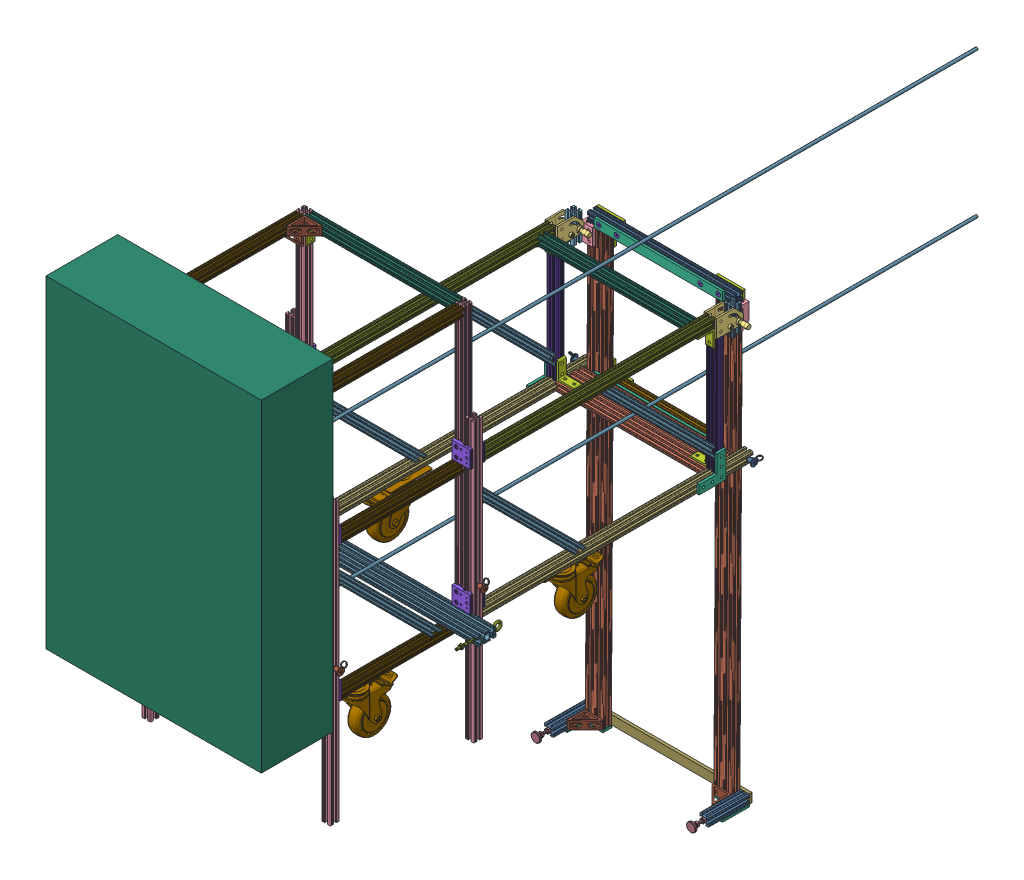
SolidWorks assembly _Tow System Assy V1.1, configuration Default. Lengths in mm. (continued)
Mates (geometry in assembly coordinates): (continued)
- Coincident1147: coincident aligned: plane of 8020 -1inch - 2 ft 3 in-13 through (-9.5504 12.7 -901.7) normal (0 1 0); plane of 8020 -1inch - 1 ft 3 in-2 through (-6.3331 12.7 190.5) normal (0 1 0)
- Coincident1148: coincident aligned: plane of 8020 -1inch - 2 ft 8 inches-1 through (-9.5504 -393.7 -215.9) normal (0 -1 0); plane of 8020 -1inch - 2 ft 7 inches-1 through (6.4164 -393.7 -212.6098) normal (0 -1 0)
- Coincident1149: coincident aligned: plane of 8020 -1inch - 2 ft 8 inches-1 through (-12.7 -371.4496 -215.9) normal (-1 0 0); plane of 8020 -1inch - 2 ft 7 inches-1 through (-12.7 393.7 -212.7504) normal (-1 0 0)
- Coincident1153: coincident anti-aligned: plane of 8020 -1inch - 1 ft 4.75 in-9 through (438.15 -374.6669 190.5) normal (0 0 -1); plane of 8020 -1inch - 1 ft 3 in-3 through (-6.4164 -390.4098 190.5) normal (0 0 1)
- Coincident1154: coincident anti-aligned: plane of 8020 -1inch - 1 ft 4.75 in-9 through (12.7 -374.5836 212.6098) normal (-1 0 0); plane of 8020 -1inch - 1 ft 3 in-3 through (12.7 -374.6669 190.5) normal (1 0 0)
- Coincident1158: coincident anti-aligned: plane of 8020 -1inch - 2 ft 8 inches-1 through (-6.4164 -390.4098 -215.9) normal (0 0 1); plane of 8020 -1inch - 2 ft 7 inches-1 through (-6.3331 393.7 -215.9) normal (0 0 -1)
- Coincident1159: coincident: plane of 8020 -1inch - 1 ft 3 in-3 through (-12.7 -371.4496 190.5) normal (-1 0 0); line of 8020 -1inch - 2 ft 8 inches-1 through (-12.7 -371.4496 -215.9) axis (0 0 -1)
- Coincident1161: coincident aligned: plane of 8020 -1inch - 2 ft 3 in-13 through (-12.7 6.3331 -901.7) normal (-1 0 0); plane of 47065T701_45 Brace - 18 in-1 through (-12.7 -47.2378 -213.673) normal (-1 0 0)
- Coincident1162: coincident aligned: plane of 8020 -1inch - 2 ft 3 in-13 through (-12.7 6.3331 -901.7) normal (-1 0 0); plane of 8020 -1inch - 1 ft 3 in-2 through (-12.7 9.5504 190.5) normal (-1 0 0)
- Coincident1164: coincident anti-aligned: plane of 47065T512_8020 - 3inch - 1 ft 4.75 in-1 through (12.7 -370.9416 -901.7) normal (-1 0 0); plane of 8020 -1inch - 2 ft 8 inches-1 through (12.7 -374.6669 -215.9) normal (1 0 0)
- Coincident1165: coincident aligned: plane of 8020 -1inch - 2 ft 3 in-13 through (6.4164 -9.4098 -215.9) normal (0 0 1); plane of 8020 -1inch - 2 ft 3 in-14 through (457.2664 -9.4098 -215.9) normal (0 0 1)
- Coincident1166: coincident aligned: plane of 8020 -1inch - 1 ft 3 in-3 through (-9.5504 -393.7 190.5) normal (0 -1 0); plane of 8020 -1inch - 2 ft 7 inches-2 through (6.4164 -393.7 193.7902) normal (0 -1 0)
- Coincident1167: coincident aligned: plane of 8020 -1inch - 1 ft 4.75 in-9 through (438.15 -387.3331 215.9) normal (0 0 1); plane of 8020 -1inch - 2 ft 7 inches-2 through (-9.5504 393.7 215.9) normal (0 0 1)
- Coincident1168: coincident anti-aligned: plane of 8020 -1inch - 1 ft 4.75 in-9 through (12.7 -374.5836 212.6098) normal (-1 0 0); plane of 8020 -1inch - 2 ft 7 inches-2 through (12.7 393.7 212.7504) normal (1 0 0)
- Coincident1169: coincident anti-aligned: plane of 47065T701_45 Brace - 18 in-1 through (-12.7 -80.9316 -215.9) normal (0 0 1); plane of 8020 -1inch - 2 ft 7 inches-1 through (-6.3331 393.7 -215.9) normal (0 0 -1)
- Coincident1170: coincident anti-aligned: plane of 8020 - 2inch - 1 ft 4.75 in-9 through (12.7 239.7749 190.5) normal (-1 0 0); plane of 8020 -1inch - 2 ft 7 inches-2 through (12.7 393.7 212.7504) normal (1 0 0)
- Coincident1171: coincident aligned: plane of 8020 - 2inch - 1 ft 4.75 in-9 through (438.15 280.5504 215.9) normal (0 0 1); plane of 8020 -1inch - 2 ft 7 inches-2 through (6.3331 393.7 215.9) normal (0 0 1)
- Coincident1175: coincident anti-aligned: plane of 8020 -1inch - 2 ft 7 inches-2 through (12.7 393.7 212.7504) normal (1 0 0); plane of 8020 - 2inch - 1 ft 4.75 in-12 through (12.7 163.5749 190.5) normal (-1 0 0)
- Coincident1176: coincident aligned: plane of 8020 -1inch - 2 ft 7 inches-2 through (6.3331 393.7 215.9) normal (0 0 1); plane of 8020 - 2inch - 1 ft 4.75 in-12 through (438.15 204.3504 215.9) normal (0 0 1)
- Coincident1178: coincident aligned: plane of 8020 -1inch - 1 ft 3 in-2 through (-6.4164 -9.4098 -190.5) normal (0 0 -1); plane of 8020 -1inch - 1 ft 3 in-3 through (-6.4164 -390.4098 -190.5) normal (0 0 -1)
- Coincident1179: coincident anti-aligned: plane of 8020 -1inch - 2 ft 7 inches-1 through (-9.5504 393.7 -190.5) normal (0 0 1); plane of 8020 -1inch - 1 ft 3 in-7 through (-6.4164 371.5902 -190.5) normal (0 0 -1)
- Coincident1180: coincident aligned: plane of 8020 -1inch - 2 ft 7 inches-1 through (-12.7 393.7 -196.8669) normal (-1 0 0); plane of 8020 -1inch - 1 ft 3 in-7 through (-12.7 390.5504 190.5) normal (-1 0 0)
- Coincident1181: coincident aligned: plane of 8020 -1inch - 2 ft 7 inches-1 through (6.4164 393.7 -212.6098) normal (0 1 0); plane of 8020 -1inch - 1 ft 3 in-7 through (-6.3331 393.7 190.5) normal (0 1 0)
- Coincident1182: coincident: plane of 8020 -1inch - 1 ft 3 in-3 through (-12.7 -371.4496 190.5) normal (-1 0 0); line of 47065T701_45 Brace - 18 in-11 through (-12.7 -54.0147 190.5) axis (0 -0.707107 -0.707107)
- Coincident1183: coincident anti-aligned: plane of 8020 -1inch - 2 ft 7 inches-2 through (-6.3331 393.7 190.5) normal (0 0 -1); plane of 47065T701_45 Brace - 18 in-11 through (-12.7 -80.9316 190.5) normal (0 0 1)
- Coincident1184: coincident anti-aligned: plane of 8020 -1inch - 1 ft 3 in-3 through (-6.3331 -368.3 190.5) normal (0 1 0); plane of 47065T701_45 Brace - 18 in-11 through (-12.7 -368.3 -96.8684) normal (0 -1 0)
- Coincident1189: coincident anti-aligned: plane of 47065T701_45 Brace - 18 in-10 through (-12.7 300.0684 190.5) normal (0 0 1); plane of 8020 -1inch - 2 ft 7 inches-2 through (-6.3331 393.7 190.5) normal (0 0 -1)
- Coincident1190: coincident anti-aligned: plane of 1 inch x 2 inch L bracket-10 through (63.5 368.3 -215.9) normal (0 1 0); plane of 8020 -1inch - 1 ft 3 in-7 through (6.3331 368.3 190.5) normal (0 -1 0)
- Coincident1191: coincident aligned: plane of 1 inch x 2 inch L bracket-10 through (12.7 322.2752 -215.9) normal (0 0 -1); plane of 8020 -1inch - 2 ft 7 inches-1 through (9.5504 393.7 -215.9) normal (0 0 -1)
- Coincident1192: coincident anti-aligned: plane of 1 inch x 2 inch L bracket-10 through (12.7 368.3 -215.9) normal (-1 0 0); plane of 8020 -1inch - 2 ft 7 inches-1 through (12.7 393.7 -209.5331) normal (1 0 0)
- Coincident1198: coincident aligned: plane of 8020 -1inch - 1 ft 3 in-2 through (-6.3331 12.7 190.5) normal (0 1 0); plane of T Bracket-25 through (19.05 12.7 190.5) normal (0 1 0)
- Coincident1199: coincident: line of 8020 -1inch - 1 ft 3 in-7 through (-6.3331 393.7 190.5) axis (0 0 -1); plane of L Bracket-19 through (12.7 393.7 222.25) normal (0 1 0)
- Coincident1200: coincident aligned: plane of 8020 -1inch - 1 ft 3 in-7 through (-12.7 390.5504 190.5) normal (-1 0 0); plane of L Bracket-19 through (-12.7 393.7 222.25) normal (-1 0 0)
- Coincident1201: coincident anti-aligned: plane of 8020 -1inch - 2 ft 7 inches-2 through (-9.5504 393.7 215.9) normal (0 0 1); plane of L Bracket-19 through (63.5 381 215.9) normal (0 0 -1)
- Coincident1204: coincident anti-aligned: plane of 8020 -1inch - 2 ft 3 in-13 through (-9.5504 12.7 -901.7) normal (0 1 0); plane of 47065T778_1 in Slider-1 through (12.7 12.7 -223.8248) normal (0 -1 0)
- Coincident1208: coincident aligned: plane of T Bracket-17 through (12.7 -393.7 -165.1) normal (0 -1 0); plane of 8020 -1inch - 2 ft 8 inches-1 through (-9.5504 -393.7 -215.9) normal (0 -1 0)
- Coincident1209: coincident anti-aligned: plane of T Bracket-17 through (12.7 -368.3 -215.9) normal (0 0 -1); plane of 8020 -1inch - 2 ft 8 inches-1 through (-6.4164 -390.4098 -215.9) normal (0 0 1)
- Coincident1212: coincident anti-aligned: plane of 47065T778_1 in Slider-1 through (-33.4772 60.198 -216.0524) normal (0 0 1); plane of 8020 -1inch - 2 ft 7 inches-3 through (-35.5431 126.825 -216.0524) normal (0 0 -1)
- Coincident1213: coincident anti-aligned: plane of 47065T778_1 in Slider-1 through (-16.51 12.7 -199.3138) normal (-1 0 0); plane of 8020 -1inch - 2 ft 7 inches-3 through (-16.51 126.825 -193.802) normal (1 0 0)
- Coincident1216: coincident aligned: plane of 8020 - 2inch - 1 ft 4.75 in-10 through (12.7 -171.2251 190.5) normal (-1 0 0); plane of 8020 - 2inch - 1 ft 4.75 in-11 through (12.7 -247.4251 190.5) normal (-1 0 0)
- Coincident1217: coincident anti-aligned: plane of T Bracket-17 through (12.7 -317.5 -203.2) normal (-1 0 0); plane of 8020 -1inch - 2 ft 7 inches-1 through (12.7 393.7 -209.5331) normal (1 0 0)
- Coincident1221: coincident anti-aligned: plane of 8020 -1inch - 1 ft 2 in-1 through (-12.7 -12.7 -923.9504) normal (-1 0 0); plane of L Bracket-17 through (-12.7 -317.5 -914.4) normal (1 0 0)
- Coincident1222: coincident aligned: plane of 8020 -1inch - 1 ft 2 in-1 through (-9.5504 -12.7 -901.7) normal (0 0 1); plane of L Bracket-17 through (-19.05 -317.5 -901.7) normal (0 0 1)
- Coincident1223: coincident aligned: plane of L Bracket-17 through (-19.05 -368.3 -851.3) normal (0 1 0); plane of 8020 -1inch - 2 ft 8 inches-1 through (-6.3331 -368.3 -215.9) normal (0 1 0)
- Coincident1224: coincident aligned: line of 8020 -1inch - 1 ft 3 in-3 through (-6.3331 -368.3 190.5) axis (0 0 -1); line of 8020 -1inch - 2 ft 8 inches-1 through (-6.3331 -368.3 -215.9) axis (0 0 -1)
- Coincident1225: coincident aligned: plane of 8020 -1inch - 2 ft 3 in-13 through (6.4164 -9.4098 -215.9) normal (0 0 1); plane of 8020 -1inch - 2 ft 8 inches-2 through (444.4336 -390.4098 -215.9) normal (0 0 1)
- Coincident1226: coincident anti-aligned: plane of 47065T701_45 Brace - 18 in-2 through (438.15 -368.3 -96.8684) normal (0 -1 0); plane of 8020 -1inch - 2 ft 8 inches-2 through (460.4004 -368.3 -215.9) normal (0 1 0)
- Coincident1227: coincident anti-aligned: plane of 8020 -1inch - 1 ft 3 in-2 through (12.7 6.3331 190.5) normal (1 0 0); plane of T Bracket-25 through (12.7 0 139.7) normal (-1 0 0)
- Coincident1228: coincident aligned: plane of 8020 -1inch - 2 ft 7 inches-2 through (9.5504 393.7 190.5) normal (0 0 -1); plane of T Bracket-25 through (19.05 38.1 190.5) normal (0 0 -1)
- Coincident1230: coincident anti-aligned: plane of 8020 -1inch - 1 ft 3 in-3 through (12.7 -374.6669 190.5) normal (1 0 0); plane of 47065T736_ Interior 90 guesset for 1 in-3 through (12.7 -390.525 190.5) normal (-1 0 0)
- Coincident1231: coincident anti-aligned: plane of 8020 -1inch - 1 ft 4.75 in-9 through (438.15 -374.6669 190.5) normal (0 0 -1); plane of 47065T736_ Interior 90 guesset for 1 in-3 through (63.5 -390.525 190.5) normal (0 0 1)
- Coincident1232: coincident aligned: plane of 8020 -1inch - 1 ft 4.75 in-9 through (438.15 -368.3 193.6496) normal (0 1 0); plane of 47065T736_ Interior 90 guesset for 1 in-3 through (15.4972 -368.3 144.4752) normal (0 1 0)
- Coincident1233: coincident aligned: plane of 8020 - 2inch - 1 ft 4.75 in-10 through (438.15 -155.8496 215.9) normal (0 0 1); plane of 8020 - 2inch - 1 ft 4.75 in-11 through (438.15 -206.6496 215.9) normal (0 0 1)
- Coincident1235: coincident aligned: plane of 8020 - 2inch - 1 ft 4.75 in-9 through (12.7 239.7749 190.5) normal (-1 0 0); plane of 8020 - 2inch - 1 ft 4.75 in-10 through (12.7 -171.2251 190.5) normal (-1 0 0)
- Coincident1239: coincident anti-aligned: plane of 8020 -1inch - 1 ft 3 in-2 through (-6.3331 12.7 190.5) normal (0 1 0); plane of 47065T778_1 in Slider-4 through (12.7 12.7 223.8248) normal (0 -1 0)
- Coincident1242: coincident: line of 8020 -1inch - 1 ft 3 in-3 through (-6.3331 -368.3 190.5) axis (0 0 -1); plane of 47065T778_1 in Slider-3 through (12.7 -368.3 223.8248) normal (0 -1 0)
- Coincident1243: coincident anti-aligned: plane of 8020 -1inch - 2 ft 7 inches-5 through (-38.7604 126.825 216.0524) normal (0 0 1); plane of 47065T778_1 in Slider-4 through (-33.4772 12.827 216.0524) normal (0 0 -1)
- Coincident1244: coincident anti-aligned: plane of 8020 -1inch - 2 ft 7 inches-5 through (-16.51 126.825 212.9028) normal (1 0 0); plane of 47065T778_1 in Slider-4 through (-16.51 12.7 193.2686) normal (-1 0 0)
- Coincident1245: coincident aligned: plane of 8020 -1inch - 2 ft 7 inches-3 through (-22.7936 126.825 -212.7622) normal (0 1 0); plane of 8020 -1inch - 2 ft 7 inches-5 through (-22.7936 126.825 193.9426) normal (0 1 0)
- Coincident1247: coincident anti-aligned: plane of 8020 -1inch - 2 ft 7 inches-1 through (-9.5504 393.7 -190.5) normal (0 0 1); plane of 47065T736_ Interior 90 guesset for 1 in-4 through (-12.7 368.3 -190.5) normal (0 0 -1)
- Coincident1248: coincident anti-aligned: plane of 8020 -1inch - 1 ft 3 in-7 through (-9.5504 368.3 190.5) normal (0 -1 0); plane of 47065T736_ Interior 90 guesset for 1 in-4 through (-12.7 368.3 -139.7) normal (0 1 0)
- Coincident1249: coincident aligned: plane of 8020 -1inch - 1 ft 3 in-7 through (-12.7 374.6669 190.5) normal (-1 0 0); plane of 47065T736_ Interior 90 guesset for 1 in-4 through (-12.7 322.2752 -187.7028) normal (-1 0 0)
- Distance48: distance = 140 mm aligned: plane of 8020 - 2inch - 1 ft 4.75 in-10 through (438.15 -127.3 193.6496) normal (0 1 0); plane of 8020 -1inch - 2 ft 3 in-14 through (441.2996 12.7 -901.7) normal (0 1 0)
- Coincident1252: coincident aligned: plane of 8020 -1inch - 2 ft 3 in-14 through (463.55 9.5504 -901.7) normal (1 0 0); plane of 8020 -1inch - 1 ft 3 in-6 through (463.55 6.3331 190.5) normal (1 0 0)
- Coincident1255: coincident: plane of 8020 -1inch - 1 ft 3 in-3 through (-6.4164 -390.4098 -190.5) normal (0 0 -1); line of 8020 -1inch - 2 ft 7 inches-1 through (-9.5504 393.7 -190.5) axis (0 -1 0)
- Coincident1256: coincident anti-aligned: plane of 8020 -1inch - 1 ft 4.75 in-9 through (438.15 -374.6669 190.5) normal (0 0 -1); plane of 8020 -1inch - 1 ft 3 in-4 through (444.4336 -390.4098 190.5) normal (0 0 1)
- Coincident1257: coincident anti-aligned: plane of 8020 -1inch - 1 ft 4.75 in-9 through (438.15 -374.5836 212.6098) normal (1 0 0); plane of 8020 -1inch - 1 ft 3 in-4 through (438.15 -371.4496 190.5) normal (-1 0 0)
- Coincident1258: coincident aligned: plane of 8020 -1inch - 1 ft 3 in-4 through (444.4336 -390.4098 190.5) normal (0 0 1); plane of 8020 -1inch - 1 ft 3 in-6 through (444.4336 -9.4098 190.5) normal (0 0 1)
- Coincident1260: coincident aligned: plane of 8020 -1inch - 1 ft 3 in-4 through (463.55 -374.6669 190.5) normal (1 0 0); plane of 8020 -1inch - 2 ft 8 inches-2 through (463.55 -374.6669 -215.9) normal (1 0 0)
- Coincident1261: coincident: line of 8020 -1inch - 1 ft 3 in-4 through (463.55 -371.4496 190.5) axis (0 0 -1); plane of 47065T701_45 Brace - 18 in-2 through (463.55 -60.7441 206.2333) normal (1 0 0)
- Coincident1262: coincident aligned: plane of 8020 -1inch - 1 ft 3 in-4 through (444.4336 -390.4098 190.5) normal (0 0 1); plane of 47065T701_45 Brace - 18 in-2 through (438.15 -80.9316 190.5) normal (0 0 1)
- Coincident1263: coincident aligned: plane of 8020 -1inch - 2 ft 3 in-14 through (457.1831 12.7 -901.7) normal (0 1 0); plane of 8020 -1inch - 1 ft 3 in-6 through (460.4004 12.7 190.5) normal (0 1 0)
- Coincident1265: coincident: line of 8020 -1inch - 2 ft 8 inches-2 through (463.55 -371.4496 -215.9) axis (0 0 -1); plane of 47065T701_45 Brace - 18 in-12 through (463.55 -49.5128 -211.398) normal (1 0 0)
- Coincident1266: coincident anti-aligned: plane of 8020 -1inch - 2 ft 8 inches-2 through (460.4004 -368.3 -215.9) normal (0 1 0); plane of 47065T701_45 Brace - 18 in-12 through (438.15 -368.3 -503.2684) normal (0 -1 0)
- Coincident1267: coincident aligned: plane of 8020 -1inch - 2 ft 8 inches-2 through (444.4336 -390.4098 -215.9) normal (0 0 1); plane of 47065T701_45 Brace - 18 in-12 through (438.15 -80.9316 -215.9) normal (0 0 1)
- Distance49: distance = 110 mm aligned: plane of 8020 - 2inch - 1 ft 4.75 in-9 through (438.15 283.7 209.5331) normal (0 1 0); plane of 8020 -1inch - 2 ft 7 inches-2 through (6.4164 393.7 193.7902) normal (0 1 0)
- Coincident1269: coincident anti-aligned: plane of 8020 -1inch - 1 ft 3 in-7 through (12.7 387.3331 190.5) normal (1 0 0); plane of 8020 -1inch - 1 ft 4.75 in-20 through (12.7 387.4164 212.6098) normal (-1 0 0)
- Coincident1270: coincident aligned: plane of 8020 -1inch - 1 ft 3 in-7 through (9.5504 393.7 190.5) normal (0 1 0); plane of 8020 -1inch - 1 ft 4.75 in-20 through (438.15 393.7 209.5331) normal (0 1 0)
- Coincident1272: coincident anti-aligned: plane of 8020 -1inch - 1 ft 3 in-7 through (-6.4164 371.5902 190.5) normal (0 0 1); plane of 8020 -1inch - 1 ft 4.75 in-20 through (438.15 387.3331 190.5) normal (0 0 -1)
- Coincident1273: coincident anti-aligned: plane of 8020 -1inch - 1 ft 3 in-7 through (-6.4164 371.5902 -190.5) normal (0 0 -1); plane of 8020 -1inch - 1 ft 4.75 in-19 through (438.15 390.5504 -190.5) normal (0 0 1)
- Coincident1274: coincident aligned: plane of 8020 -1inch - 1 ft 3 in-7 through (9.5504 393.7 190.5) normal (0 1 0); plane of 8020 -1inch - 1 ft 4.75 in-19 through (438.15 393.7 -196.8669) normal (0 1 0)
- Coincident1275: coincident anti-aligned: plane of 8020 -1inch - 1 ft 3 in-7 through (12.7 387.3331 190.5) normal (1 0 0); plane of 8020 -1inch - 1 ft 4.75 in-19 through (12.7 387.4164 -193.7902) normal (-1 0 0)
- Coincident1276: coincident anti-aligned: plane of 8020 -1inch - 1 ft 2 in-2 through (463.55 -12.7 -904.8496) normal (1 0 0); plane of L Bracket-18 through (463.55 -381 -850.9) normal (-1 0 0)
- Coincident1277: coincident aligned: plane of 8020 -1inch - 2 ft 8 inches-2 through (460.4004 -368.3 -215.9) normal (0 1 0); plane of L Bracket-18 through (469.9 -368.3 -850.9) normal (0 1 0)
- Coincident1278: coincident anti-aligned: plane of 47065T512_8020 - 3inch - 1 ft 4.75 in-1 through (12.7 -368.3 -904.8496) normal (0 1 0); plane of 1 inch x 2 inch L bracket-44 through (63.5 -368.3 -904.875) normal (0 -1 0)
- Coincident1279: coincident anti-aligned: plane of 47065T512_8020 - 3inch - 1 ft 4.75 in-1 through (12.7 -368.3 -904.8496) normal (0 1 0); plane of 1 inch x 2 inch L bracket-45 through (387.35 -368.3 -927.1) normal (0 -1 0)
- Coincident1280: coincident anti-aligned: plane of 8020 -1inch - 1 ft 3 in-7 through (12.7 387.3331 190.5) normal (1 0 0); plane of 47065T736_ Interior 90 guesset for 1 in-5 through (12.7 371.475 -139.7) normal (-1 0 0)
- Coincident1281: coincident aligned: plane of 8020 -1inch - 1 ft 3 in-7 through (-6.3331 393.7 190.5) normal (0 1 0); plane of 47065T736_ Interior 90 guesset for 1 in-5 through (58.7248 393.7 -187.7028) normal (0 1 0)
- Coincident1282: coincident anti-aligned: plane of 8020 -1inch - 1 ft 4.75 in-19 through (438.15 390.5504 -190.5) normal (0 0 1); plane of 47065T736_ Interior 90 guesset for 1 in-5 through (12.7 371.475 -190.5) normal (0 0 -1)
- Coincident1283: coincident aligned: plane of 8020 -1inch - 2 ft 7 inches-1 through (6.4164 393.7 -212.6098) normal (0 1 0); plane of 8020 -1inch - 2 ft 7 inches-6 through (457.2664 393.7 -212.6098) normal (0 1 0)
- Coincident1284: coincident: line of 8020 -1inch - 2 ft 7 inches-1 through (-6.3331 393.7 -215.9) axis (0 -1 0); plane of 8020 -1inch - 2 ft 7 inches-6 through (444.5169 393.7 -215.9) normal (0 0 -1)
- Coincident1285: coincident anti-aligned: plane of 8020 -1inch - 1 ft 4.75 in-19 through (438.15 387.4164 -193.7902) normal (1 0 0); plane of 8020 -1inch - 2 ft 7 inches-6 through (438.15 393.7 -212.7504) normal (-1 0 0)
- Coincident1286: coincident aligned: plane of 8020 -1inch - 2 ft 7 inches-6 through (457.2664 393.7 -212.6098) normal (0 1 0); plane of 8020 -1inch - 2 ft 7 inches-8 through (457.2664 393.7 193.7902) normal (0 1 0)
- Coincident1287: coincident aligned: plane of 8020 -1inch - 2 ft 7 inches-6 through (463.55 393.7 -209.5331) normal (1 0 0); plane of 8020 -1inch - 2 ft 7 inches-8 through (463.55 393.7 196.8669) normal (1 0 0)
- Coincident1288: coincident aligned: plane of 8020 -1inch - 1 ft 4.75 in-20 through (438.15 387.3331 190.5) normal (0 0 -1); plane of 8020 -1inch - 2 ft 7 inches-8 through (444.5169 393.7 190.5) normal (0 0 -1)
- Coincident1289: coincident aligned: plane of 8020 -1inch - 1 ft 4.75 in-20 through (438.15 393.7 193.6496) normal (0 1 0); plane of 8020 -1inch - 1 ft 3 in-8 through (444.5169 393.7 190.5) normal (0 1 0)
- Coincident1290: coincident anti-aligned: plane of 8020 -1inch - 1 ft 4.75 in-20 through (438.15 387.4164 212.6098) normal (1 0 0); plane of 8020 -1inch - 1 ft 3 in-8 through (438.15 390.5504 190.5) normal (-1 0 0)
- Coincident1291: coincident anti-aligned: plane of 8020 -1inch - 1 ft 4.75 in-20 through (438.15 387.3331 190.5) normal (0 0 -1); plane of 8020 -1inch - 1 ft 3 in-8 through (444.4336 371.5902 190.5) normal (0 0 1)
- Coincident1294: coincident anti-aligned: plane of 8020 -1inch - 2 ft 3 in-14 through (457.1831 12.7 -901.7) normal (0 1 0); plane of 47065T778_1 in Slider-6 through (438.15 12.7 -223.8248) normal (0 -1 0)
- Coincident1301: coincident anti-aligned: plane of 8020 -1inch - 1 ft 3 in-6 through (460.4004 12.7 190.5) normal (0 1 0); plane of 47065T778_1 in Slider-8 through (438.15 12.7 182.5752) normal (0 -1 0)
- Coincident1304: coincident anti-aligned: plane of 8020 -1inch - 1 ft 3 in-4 through (460.4004 -368.3 190.5) normal (0 1 0); plane of 47065T778_1 in Slider-7 through (438.15 -368.3 223.8248) normal (0 -1 0)
- Coincident1305: coincident anti-aligned: plane of 8020 -1inch - 2 ft 7 inches-7 through (470.5096 126.825 216.0524) normal (0 0 1); plane of 47065T778_1 in Slider-8 through (484.3272 60.198 216.0524) normal (0 0 -1)
- Coincident1306: coincident anti-aligned: plane of 8020 -1inch - 2 ft 7 inches-7 through (467.36 126.825 209.6855) normal (-1 0 0); plane of 47065T778_1 in Slider-8 through (467.36 12.7 213.1314) normal (1 0 0)
- Coincident1307: coincident aligned: plane of 8020 -1inch - 2 ft 7 inches-5 through (-22.7936 126.825 193.9426) normal (0 1 0); plane of 8020 -1inch - 2 ft 7 inches-7 through (486.4764 126.825 193.9426) normal (0 1 0)
- Coincident1308: coincident anti-aligned: plane of 47065T778_1 in Slider-6 through (484.3272 60.198 -190.3476) normal (0 0 -1); plane of 8020 -1inch - 2 ft 7 inches-9 through (470.5096 126.825 -190.3476) normal (0 0 1)
- Coincident1309: coincident anti-aligned: plane of 47065T778_1 in Slider-6 through (467.36 12.7 -193.2686) normal (1 0 0); plane of 8020 -1inch - 2 ft 7 inches-9 through (467.36 126.825 -196.7145) normal (-1 0 0)
- Coincident1310: coincident aligned: plane of 8020 -1inch - 2 ft 7 inches-7 through (486.4764 126.825 193.9426) normal (0 1 0); plane of 8020 -1inch - 2 ft 7 inches-9 through (486.4764 126.825 -212.4574) normal (0 1 0)
- Coincident1313: coincident aligned: plane of 8020 -1inch - 1 ft 3 in-2 through (0 0 0) normal (0 0 1)
- Coincident1314: coincident aligned: plane of 8020 -1inch - 1 ft 3 in-2 through (0 0 0) normal (0 1 0)
- Coincident1315: coincident aligned: plane of 8020 -1inch - 1 ft 3 in-2 through (0 0 0) normal (1 0 0)
- Coincident1316: coincident aligned: plane of 8020 -1inch - 415mm-1 through (433.1224 9.4721 -1008.3493) normal (0 0.999985 -0.005452); plane of T Bracket-24 through (94.3224 9.4203 -1017.8488) normal (0 0.999985 -0.005452)
- Coincident1317: coincident aligned: plane of 8020 -1inch - 415mm-1 through (433.1224 9.4721 -1008.3493) normal (0 0.999985 -0.005452); plane of T Bracket-23 through (432.7276 9.4203 -1017.8488) normal (0 0.999985 -0.005452)
- Coincident1318: coincident aligned: plane of 47065T125_2inch - 4 ft-1 through (18.1224 -15.9275 -1008.2108) normal (-1 0 0); plane of 8020 -1inch - 415mm-1 through (18.1224 -12.5503 -992.2622) normal (-1 0 0)
- Coincident1321: coincident anti-aligned: plane of T Bracket-25 through (19.05 12.7 139.7) normal (0 0 -1); plane of 47065T237_8020 2 in interior corner bracket-1 through (-7.9248 20.6375 139.7) normal (0 0 1)
- Coincident1322: coincident aligned: plane of 8020 -1inch - 1 ft 3 in-2 through (12.7 -9.5504 190.5) normal (1 0 0); plane of 47065T237_8020 2 in interior corner bracket-1 through (12.7 46.0375 139.7) normal (1 0 0)
- Coincident1323: coincident anti-aligned: plane of 47065T237_8020 2 in interior corner bracket-1 through (12.7 20.6375 139.7) normal (0 -1 0); plane of 1614T644_1in x 48mm Aluminium bar - 5_16 thick-1 through (12.7 20.6375 140.075) normal (0 1 0)
- Coincident1324: coincident aligned: plane of 47065T237_8020 2 in interior corner bracket-1 through (-7.9248 20.6375 92.075) normal (0 0 -1); plane of 1614T644_1in x 48mm Aluminium bar - 5_16 thick-1 through (0 16.6687 92.075) normal (0 0 -1)
- Coincident1325: coincident aligned: plane of 47065T237_8020 2 in interior corner bracket-1 through (12.7 46.0375 139.7) normal (1 0 0); plane of 1614T644_1in x 48mm Aluminium bar - 5_16 thick-1 through (12.7 20.6375 140.075) normal (1 0 0)
- Coincident1326: coincident anti-aligned: plane of 8020 -1inch - 1 ft 3 in-2 through (9.5504 12.7 190.5) normal (0 1 0); plane of 1614T644_1in x 48mm Aluminium bar - 5_16 thick-1 through (12.7 12.7 140.075) normal (0 -1 0)
- Coincident1329: coincident aligned: plane of 8020 - 2inch - 1 ft 4.75 in-10 through (438.15 -130.4496 215.9) normal (0 0 1); plane of 8020 - 2inch - 1 ft 4.75 in-12 through (438.15 204.3504 215.9) normal (0 0 1)
- Coincident1334: coincident anti-aligned: plane of 8020 -1inch - 2 ft 8 inches-1 through (-9.5504 -393.7 -215.9) normal (0 -1 0); plane of 5537T435_ Caster Wheel 265lb Cap-1 through (-1.2 -393.7 -479.1893) normal (0 1 0)
- Coincident1335: coincident aligned: plane of 8020 -1inch - 2 ft 8 inches-1 through (-12.7 -387.3331 -215.9) normal (-1 0 0); plane of 5537T435_ Caster Wheel 265lb Cap-1 through (-12.7 -393.7 -505.2661) normal (-1 0 0)
- Coincident1336: coincident: line of 47065T701_45 Brace - 18 in-1 through (-6.3331 -368.2999 -539.1893) axis (-1 0 0); plane of 5537T435_ Caster Wheel 265lb Cap-1 through (27.3 -393.7 -539.1893) normal (0 0 -1)
- Coincident1337: coincident aligned: plane of 8020 -1inch - 1 ft 3 in-3 through (-12.7 -387.3331 190.5) normal (-1 0 0); plane of 5537T435_ Caster Wheel 265lb Cap-2 through (-12.7 -393.7 54.4232) normal (-1 0 0)
- Coincident1338: coincident anti-aligned: plane of 8020 -1inch - 1 ft 3 in-3 through (-9.5504 -393.7 190.5) normal (0 -1 0); plane of 5537T435_ Caster Wheel 265lb Cap-2 through (-1.2 -393.7 80.5) normal (0 1 0)
- Distance51: distance = 50 mm aligned: plane of 5537T435_ Caster Wheel 265lb Cap-2 through (27.3 -393.7 140.5) normal (0 0 1); plane of 8020 -1inch - 1 ft 3 in-3 through (-6.4164 -390.4098 190.5) normal (0 0 1)
- Coincident1340: coincident anti-aligned: plane of 8020 -1inch - 1 ft 3 in-4 through (457.1831 -393.7 190.5) normal (0 -1 0); plane of 5537T435_ Caster Wheel 265lb Cap-4 through (452.05 -393.7 105.1) normal (0 1 0)
- Coincident1341: coincident anti-aligned: plane of 8020 -1inch - 2 ft 8 inches-2 through (457.1831 -393.7 -215.9) normal (0 -1 0); plane of 5537T435_ Caster Wheel 265lb Cap-3 through (452.05 -393.7 -479.1893) normal (0 1 0)
- Coincident1342: coincident aligned: plane of 8020 -1inch - 2 ft 8 inches-2 through (463.55 -374.6669 -215.9) normal (1 0 0); plane of 5537T435_ Caster Wheel 265lb Cap-3 through (463.55 -393.7 -539.1893) normal (1 0 0)
- Coincident1343: coincident: line of 47065T701_45 Brace - 18 in-12 through (460.4004 -368.2999 -539.1893) axis (-1 0 0); plane of 5537T435_ Caster Wheel 265lb Cap-3 through (423.55 -393.7 -539.1893) normal (0 0 -1)
- Coincident1344: coincident aligned: plane of 8020 -1inch - 1 ft 3 in-4 through (463.55 -390.5504 190.5) normal (1 0 0); plane of 5537T435_ Caster Wheel 265lb Cap-4 through (463.55 -393.7 131.1768) normal (1 0 0)
- Distance52: distance = 25.4 mm anti-aligned: plane of 5537T435_ Caster Wheel 265lb Cap-4 through (423.55 -393.7 165.1) normal (0 0 1); plane of 8020 -1inch - 2 ft 7 inches-8 through (460.4004 393.7 190.5) normal (0 0 -1)
- Distance55: distance = 25.4 mm anti-aligned: plane of L Bracket-19 through (63.5 381 222.25) normal (0 0 1); plane of Electrical Enclosure Placeholder-1 through (-77.7 -393.7 247.65) normal (0 0 -1)
- Coincident1348: coincident aligned: plane of 8020 -1inch - 1 ft 4.75 in-9 through (438.15 -393.7 212.7504) normal (0 -1 0); plane of Electrical Enclosure Placeholder-1 through (-77.7 -393.7 450.85) normal (0 -1 0)
- Distance53: distance = 65 mm aligned: plane of Electrical Enclosure Placeholder-1 through (-77.7 -393.7 450.85) normal (-1 0 0); plane of 8020 -1inch - 2 ft 7 inches-2 through (-12.7 393.7 209.5331) normal (-1 0 0)
- Concentric49: concentric anti-aligned: cylinder of 8020 -1inch - 2 ft 7 inches-2 through (12.7 -279.4 203.2) axis (-1 0 0) radius 3.175; cylinder of 92851A125_SS HIGH-TENSION PUSH-BUTTON QUICK-RELEASE PIN - 2in length-2 through (-62.5475 -279.4 203.2) axis (1 0 0) radius 3.1559
- Coincident1351: coincident anti-aligned: plane of 8020 -1inch - 2 ft 7 inches-5 through (-41.91 126.825 193.802) normal (-1 0 0); plane of 92851A125_SS HIGH-TENSION PUSH-BUTTON QUICK-RELEASE PIN - 2in length-2 through (-41.91 -275.3286 200.577) normal (1 0 0)
- Concentric50: concentric aligned: cylinder of 8020 -1inch - 2 ft 7 inches-6 through (463.55 -279.4 -203.2) axis (-1 0 0) radius 3.175; cylinder of 92851A125_SS HIGH-TENSION PUSH-BUTTON QUICK-RELEASE PIN - 2in length-4 through (513.3975 -279.4 -203.2) axis (-1 0 0) radius 3.1559
- Coincident1353: coincident anti-aligned: plane of 8020 -1inch - 2 ft 7 inches-9 through (492.76 126.825 -209.3807) normal (1 0 0); plane of 92851A125_SS HIGH-TENSION PUSH-BUTTON QUICK-RELEASE PIN - 2in length-4 through (492.76 -283.9092 -201.4325) normal (-1 0 0)
- Concentric51: concentric aligned: cylinder of 8020 -1inch - 2 ft 7 inches-8 through (463.55 -279.4 203.2) axis (-1 0 0) radius 3.175; cylinder of 92851A125_SS HIGH-TENSION PUSH-BUTTON QUICK-RELEASE PIN - 2in length-3 through (513.3975 -279.4 203.2) axis (-1 0 0) radius 3.1559
- Coincident1354: coincident anti-aligned: plane of 8020 -1inch - 2 ft 7 inches-7 through (492.76 126.825 197.0193) normal (1 0 0); plane of 92851A125_SS HIGH-TENSION PUSH-BUTTON QUICK-RELEASE PIN - 2in length-3 through (492.76 -283.325 206.0374) normal (-1 0 0)
- Coincident1355: coincident anti-aligned: plane of 8020 -1inch - 2 ft 7 inches-3 through (-41.91 126.825 -212.9028) normal (-1 0 0); plane of 92851A125_SS HIGH-TENSION PUSH-BUTTON QUICK-RELEASE PIN - 2in length-1 through (-41.91 -277.9317 -198.5847) normal (1 0 0)
- Coincident1356: coincident anti-aligned: plane of 8020 -1inch - 2 ft 7 inches-1 through (6.3331 393.7 -190.5) normal (0 0 1); plane of 8020 - 2inch - 2 ft 2 in-1 through (-104.775 -346.0496 -190.5) normal (0 0 -1)
- Coincident1357: coincident anti-aligned: plane of 8020 -1inch - 1 ft 3 in-3 through (-6.3331 -368.3 190.5) normal (0 1 0); plane of 8020 - 2inch - 2 ft 2 in-1 through (-104.775 -368.3 -187.3504) normal (0 -1 0)
- Concentric54: concentric aligned: cylinder of 8020 - 2inch - 2 ft 2 in-1 through (542.925 -355.6 -139.7) axis (0 0 -1) radius 4.445; cylinder of 3032T610_316 SS EYEBOLT W NUT 1-4_20 x 4 in-1 through (542.925 -355.6 -88.9) axis (0 0 -1) radius 3.175
- Coincident1363: coincident anti-aligned: plane of 8020 - 2inch - 2 ft 2 in-1 through (-104.775 -346.0496 -190.5) normal (0 0 -1); plane of 3032T610_316 SS EYEBOLT W NUT 1-4_20 x 4 in-1 through (542.925 -350.8375 -190.5) normal (0 0 1)
- Parallel19: parallel aligned: plane of 8020 - 2inch - 2 ft 2 in-1 through (-104.775 -342.9 -142.8496) normal (0 1 0); plane of 3032T610_316 SS EYEBOLT W NUT 1-4_20 x 4 in-1 through (546.1329 -350.0437 -101.6) normal (0 1 0)
- Concentric55: concentric aligned: cylinder of 8020 - 2inch - 2 ft 2 in-1 through (-92.075 -355.6 -139.7) axis (0 0 -1) radius 4.445; cylinder of 3032T610_316 SS EYEBOLT W NUT 1-4_20 x 4 in-2 through (-92.075 -355.6 -88.9) axis (0 0 -1) radius 3.175
- Coincident1365: coincident anti-aligned: plane of 8020 - 2inch - 2 ft 2 in-1 through (-104.775 -346.0496 -190.5) normal (0 0 -1); plane of 3032T610_316 SS EYEBOLT W NUT 1-4_20 x 4 in-2 through (-92.075 -350.8375 -190.5) normal (0 0 1)
- Parallel20: parallel aligned: plane of 8020 - 2inch - 2 ft 2 in-1 through (-104.775 -342.9 -142.8496) normal (0 1 0); plane of 3032T610_316 SS EYEBOLT W NUT 1-4_20 x 4 in-2 through (-88.8671 -350.0437 -101.6) normal (0 1 0)
- Coincident1367: coincident anti-aligned: plane of 8020 - 2inch - 2 ft 2 in-1 through (-104.775 -342.9 -184.1331) normal (0 1 0); plane of 47065T778_1 in Slider-2 through (12.7 -342.9 -182.5752) normal (0 -1 0)
- Coincident1368: coincident aligned: plane of 8020 - 2inch - 2 ft 2 in-1 through (225.425 -355.6 -165.1) normal (-1 0 0)
- Concentric56: concentric aligned: cylinder of 47065T125_2inch - 4 ft-1 through (18.1224 -381 -996.67) axis (1 0 0) radius 3.5; cylinder of 92851A140_SS HIGH-TENSION PUSH-BUTTON QUICK-RELEASE PIN - 4in usable length-1 through (-33.3375 -381 -996.67) axis (1 0 0) radius 3.1559
- Concentric80: concentric anti-aligned: cylinder of 8020 -1inch - 2 ft 7 inches-1 through (12.7 -279.4 -203.2) axis (-1 0 0) radius 3.175; cylinder of 92851A125_SS HIGH-TENSION PUSH-BUTTON QUICK-RELEASE PIN - 2in length-1 through (-62.5475 -279.4 -203.2) axis (1 0 0) radius 3.1559
- Distance54: distance = 66.5 mm aligned: plane of 8020 -1inch - 2 ft 7 inches-3 through (-22.7936 126.825 -212.7622) normal (0 1 0); plane of 47065T778_1 in Slider-1 through (12.7 60.325 -223.8248) normal (0 1 0)
- Coincident1369: coincident anti-aligned: plane of 8020 -1inch - 2 ft 7 inches-1 through (-6.3331 393.7 -215.9) normal (0 0 -1); plane of 47065T778_1 in Slider-2 through (-12.7 -295.275 -215.9) normal (0 0 1)
- Coincident1370: coincident aligned: plane of 8020 -1inch - 2 ft 7 inches-1 through (12.7 393.7 -209.5331) normal (1 0 0); plane of 47065T778_1 in Slider-2 through (12.7 -295.275 -215.9) normal (1 0 0)
- Coincident1371: coincident anti-aligned: plane of 8020 -1inch - 2 ft 7 inches-2 through (-6.3331 393.7 190.5) normal (0 0 -1); plane of 47065T778_1 in Slider-3 through (-12.7 -320.675 190.5) normal (0 0 1)
- Coincident1372: coincident aligned: plane of 8020 -1inch - 2 ft 7 inches-2 through (12.7 393.7 196.8669) normal (1 0 0); plane of 47065T778_1 in Slider-3 through (12.7 -320.675 190.5) normal (1 0 0)
- Coincident1373: coincident anti-aligned: plane of 8020 -1inch - 2 ft 7 inches-6 through (460.4004 393.7 -215.9) normal (0 0 -1); plane of 47065T778_1 in Slider-5 through (463.55 -342.9 -215.9) normal (0 0 1)
- Coincident1374: coincident aligned: plane of 8020 -1inch - 2 ft 7 inches-6 through (438.15 393.7 -212.7504) normal (-1 0 0); plane of 47065T778_1 in Slider-5 through (438.15 -342.9 -215.9) normal (-1 0 0)
- Coincident1376: coincident anti-aligned: plane of 8020 - 2inch - 2 ft 2 in-1 through (-104.775 -342.9 -184.1331) normal (0 1 0); plane of 47065T778_1 in Slider-5 through (438.15 -342.9 -223.8248) normal (0 -1 0)
- Coincident1377: coincident anti-aligned: plane of 8020 -1inch - 2 ft 7 inches-8 through (444.5169 393.7 190.5) normal (0 0 -1); plane of 47065T778_1 in Slider-7 through (447.7512 -368.3 190.5) normal (0 0 1)
- Coincident1378: coincident aligned: plane of 8020 -1inch - 2 ft 7 inches-8 through (438.15 393.7 193.6496) normal (-1 0 0); plane of 47065T778_1 in Slider-7 through (438.15 -368.3 190.5) normal (-1 0 0)
- Coincident1379: coincident anti-aligned: plane of 8020 -1inch - 2 ft 7 inches-1 through (-6.3331 393.7 -215.9) normal (0 0 -1); plane of 47065T778_1 in Slider-1 through (-12.7 60.325 -215.9) normal (0 0 1)
- Coincident1380: coincident aligned: plane of 8020 -1inch - 2 ft 7 inches-1 through (12.7 393.7 -209.5331) normal (1 0 0); plane of 47065T778_1 in Slider-1 through (12.7 60.325 -215.9) normal (1 0 0)
- Coincident1381: coincident anti-aligned: plane of 8020 -1inch - 2 ft 7 inches-2 through (-6.3331 393.7 190.5) normal (0 0 -1); plane of 47065T778_1 in Slider-4 through (3.0988 60.325 190.5) normal (0 0 1)
- Coincident1382: coincident aligned: plane of 8020 -1inch - 2 ft 7 inches-2 through (12.7 393.7 196.8669) normal (1 0 0); plane of 47065T778_1 in Slider-4 through (12.7 60.325 190.5) normal (1 0 0)
- Coincident1383: coincident anti-aligned: plane of 8020 -1inch - 2 ft 7 inches-8 through (457.1831 393.7 215.9) normal (0 0 1); plane of 47065T778_1 in Slider-8 through (463.55 60.325 215.9) normal (0 0 -1)
- Coincident1384: coincident aligned: plane of 8020 -1inch - 2 ft 7 inches-8 through (438.15 393.7 209.5331) normal (-1 0 0); plane of 47065T778_1 in Slider-8 through (438.15 60.325 215.9) normal (-1 0 0)
- Coincident1385: coincident anti-aligned: plane of 8020 -1inch - 2 ft 7 inches-6 through (441.2996 393.7 -190.5) normal (0 0 1); plane of 47065T778_1 in Slider-6 through (447.7512 60.325 -190.5) normal (0 0 -1)
- Coincident1386: coincident aligned: plane of 8020 -1inch - 2 ft 7 inches-6 through (438.15 393.7 -196.8669) normal (-1 0 0); plane of 47065T778_1 in Slider-6 through (438.15 60.325 -190.5) normal (-1 0 0)
- Coincident1387: coincident anti-aligned: plane of 1614T644_1in x 364mm Aluminium bar - 5_16 thick-1 through (43.5224 -393.6306 -983.901) normal (0 -0.005452 -0.999985); plane of 8020 -1inch - 1 ft 0.25-3 through (380.0724 -371.3805 -984.0223) normal (0 0.005452 0.999985)
- Coincident1389: coincident aligned: plane of 90585A358_SS Countersunk Screw 1_4-20 x 5-8 in-8 through (107.0224 -380.8981 -977.9703) normal (0 0.005452 0.999985); plane of 90585A358_SS Countersunk Screw 1_4-20 x 5-8 in-9 through (394.8224 -3.0737 -980.0301) normal (0 0.005452 0.999985)
- Coincident1390: coincident aligned: plane of 90585A358_SS Countersunk Screw 1_4-20 x 5-8 in-6 through (107.0224 -3.0737 -980.0301) normal (0 0.005452 0.999985); plane of 90585A358_SS Countersunk Screw 1_4-20 x 5-8 in-7 through (56.2224 -3.0737 -980.0301) normal (0 0.005452 0.999985)
- Coincident1391: coincident aligned: plane of 90585A358_SS Countersunk Screw 1_4-20 x 5-8 in-6 through (107.0224 -3.0737 -980.0301) normal (0 0.005452 0.999985); plane of 90585A358_SS Countersunk Screw 1_4-20 x 5-8 in-8 through (107.0224 -380.8981 -977.9703) normal (0 0.005452 0.999985)
- Coincident1392: coincident aligned: plane of 90585A358_SS Countersunk Screw 1_4-20 x 5-8 in-4 through (344.0224 -3.0737 -980.0301) normal (0 0.005452 0.999985); plane of 90585A358_SS Countersunk Screw 1_4-20 x 5-8 in-9 through (394.8224 -3.0737 -980.0301) normal (0 0.005452 0.999985)
- Coincident1393: coincident aligned: plane of 90585A358_SS Countersunk Screw 1_4-20 x 5-8 in-1 through (56.2224 -380.8981 -977.9703) normal (0 0.005452 0.999985); plane of 90585A358_SS Countersunk Screw 1_4-20 x 5-8 in-3 through (394.8224 -380.8981 -977.9703) normal (0 0.005452 0.999985)
- Coincident1394: coincident aligned: plane of 90585A358_SS Countersunk Screw 1_4-20 x 5-8 in-3 through (394.8224 -380.8981 -977.9703) normal (0 0.005452 0.999985); plane of 90585A358_SS Countersunk Screw 1_4-20 x 5-8 in-5 through (344.0224 -380.8981 -977.9703) normal (0 0.005452 0.999985)
- Coincident1395: coincident aligned: plane of 90585A358_SS Countersunk Screw 1_4-20 x 5-8 in-4 through (344.0224 -3.0737 -980.0301) normal (0 0.005452 0.999985); plane of 90585A358_SS Countersunk Screw 1_4-20 x 5-8 in-5 through (344.0224 -380.8981 -977.9703) normal (0 0.005452 0.999985)
- Concentric81: concentric aligned: circle of 1614T644_1in x 364mm Aluminium bar - 5_16 thick-2; circle of 90585A358_SS Countersunk Screw 1_4-20 x 5-8 in-9
- Concentric82: concentric aligned: circle of 1614T644_1in x 364mm Aluminium bar - 5_16 thick-2; circle of 90585A358_SS Countersunk Screw 1_4-20 x 5-8 in-4
- Concentric83: concentric aligned: circle of 1614T644_1in x 364mm Aluminium bar - 5_16 thick-2; circle of 90585A358_SS Countersunk Screw 1_4-20 x 5-8 in-6
- Concentric84: concentric aligned: circle of 1614T644_1in x 364mm Aluminium bar - 5_16 thick-2; circle of 90585A358_SS Countersunk Screw 1_4-20 x 5-8 in-7
- Concentric85: concentric aligned: circle of 1614T644_1in x 364mm Aluminium bar - 5_16 thick-1; circle of 90585A358_SS Countersunk Screw 1_4-20 x 5-8 in-8
- Concentric86: concentric aligned: circle of 1614T644_1in x 364mm Aluminium bar - 5_16 thick-1; circle of 90585A358_SS Countersunk Screw 1_4-20 x 5-8 in-1
- Concentric87: concentric aligned: circle of 1614T644_1in x 364mm Aluminium bar - 5_16 thick-1; circle of 90585A358_SS Countersunk Screw 1_4-20 x 5-8 in-3
- Concentric88: concentric aligned: circle of 1614T644_1in x 364mm Aluminium bar - 5_16 thick-1; circle of 90585A358_SS Countersunk Screw 1_4-20 x 5-8 in-5
- Coincident1396: coincident aligned: plane of 1614T644_1in x 364mm Aluminium bar - 5_16 thick-2 through (407.5224 9.6261 -980.0993) normal (0 0.005452 0.999985); plane of 90585A358_SS Countersunk Screw 1_4-20 x 5-8 in-9 through (394.8224 -3.0737 -980.0301) normal (0 0.005452 0.999985)
- Coincident1397: coincident aligned: plane of 1614T644_1in x 364mm Aluminium bar - 5_16 thick-1 through (43.5224 -393.5979 -977.901) normal (0 0.005452 0.999985); plane of 1614T644_1in x 364mm Aluminium bar - 5_16 thick-2 through (407.5224 9.6261 -980.0993) normal (0 0.005452 0.999985)
- Coincident1398: coincident aligned: plane of 1614T644_1in x 364mm Aluminium bar - 5_16 thick-2 through (407.5224 9.5934 -986.0992) normal (0 0.999985 -0.005452); plane of 8020 -1inch - 415mm-1 through (433.1224 9.5587 -992.466) normal (0 0.999985 -0.005452)
- Coincident1399: coincident aligned: plane of 1614T644_1in x 364mm Aluminium bar - 5_16 thick-1 through (43.5224 -368.231 -984.0394) normal (0 0.999985 -0.005452); plane of 8020 -1inch - 1 ft 0.25-3 through (380.0724 -368.2657 -990.4062) normal (0 0.999985 -0.005452)
- Coincident1400: coincident anti-aligned: plane of 3136N217_Heavy Duty 90 pivot-1 through (12.7 -25.4 -952.881) normal (-1 0 0); plane of 8020 -1inch - 0 ft 3 in-1 through (12.7 -63.534 -958.5899) normal (1 0 0)
- Coincident1401: coincident anti-aligned: plane of 3136N217_Heavy Duty 90 pivot-1 through (-12.7 -25.4 -927.1) normal (1 0 0); plane of 8020 -1inch - 1 ft 2 in-1 through (-12.7 -12.7 -923.9504) normal (-1 0 0)
- Coincident1402: coincident anti-aligned: plane of 3136N217_Heavy Duty 90 pivot-2 through (438.15 -25.4 -927.1) normal (1 0 0); plane of 8020 -1inch - 1 ft 2 in-2 through (438.15 -12.7 -908.0669) normal (-1 0 0)
